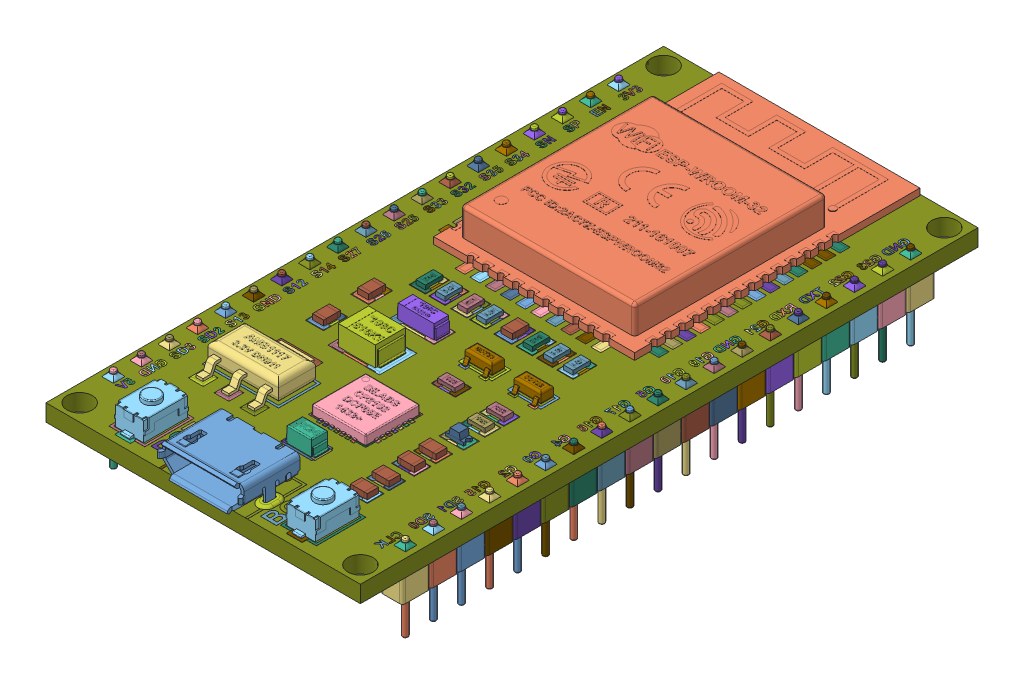
SolidWorks assembly PCB_ESP32-38Pines, configuration Default. Lengths in mm.
Overall size (28 10.12 55.48).
487 component instances, 472 part files, 0 mates.
Components (placement in the parent):
- PCB_ESP32-38Pines.step-1: PCB_ESP32-38Pines.step [Default] at origin size (28 10.12 55.48)
  - MicroUSB.step-1: MicroUSB.step [Default] at (0 2.6382 22.5) size (7.56 3.45 5.78)
  - esp32.step-1: esp32.step [Default] at (0 1.5 -14.6737) size (17.9 3.13 25.4)
  - AMS1173.3V.step-1: AMS1173.3V.step [Default] at (-6.6341 1.5 15.6567) x (-1 0 0) z (0 0 -1) size (6.3 1.81 6.45)
  - cp2102.step-1: cp2102.step [Default] at (1.1401 1.501 14.1651) x (1 0 0) z (0 1 0) size (5.1 5.1 0.81)
  - Push_Bottom.step-1: Push_Bottom.step [Default] at (-7.7988 1.5 24.2992) x (0 0 -1) z (1 0 0) size (4.7 2.2 2.7)
  - Push_Bottom.step-2: Push_Bottom.step [Default] at (7.4774 1.5 24.2992) x (0 0 -1) z (1 0 0) size (4.7 2.2 2.7)
  - Diodo_K24.step-1: Diodo_K24.step [Default] at (0.9466 1.5 19.1832) size (2.7 1.4 1.4)
  - Cap_Tam_106.step-1: Cap_Tam_106.step [Default] at (-3.6422 1.5 8.8277) size (3.8 1.81 2.7)
  - Cap_Tam_106C.step-1: Cap_Tam_106C.step [Default] at (-3.1152 1.5 4.7703) size (3.5 1.31 1.3)
  - Transistor_smd.step-1: Transistor_smd.step [Default] at (7.0469 1.5 5.1079) size (2.4 1.01 2)
  - Transistor_smd.step-2: Transistor_smd.step [Default] at (2.6755 1.5 5.1079) size (2.4 1.01 2)
  - Led_red_0603.step-1: Led_red_0603.step [Default] at (7.1609 1.5 11.8696) size (1.6 0.85 0.8)
  - Cap_0603.step-1: Cap_0603.step [Default] at (7.0673 1.5 14.1024) x (1 0 0) z (0 1 0) size (1.5 1 0.5)
  - Cap_0603.step-2: Cap_0603.step [Default] at (7.0673 1.5 16.0214) x (1 0 0) z (0 1 0) size (1.5 1 0.5)
  - Cap_0603.step-3: Cap_0603.step [Default] at (7.0673 1.5 18.2661) x (1 0 0) z (0 1 0) size (1.5 1 0.5)
  - Cap_0603.step-4: Cap_0603.step [Default] at (7.0673 2 20.2101) x (1 0 0) z (0 -1 0) size (1.5 1 0.5)
  - Res_102.step-1: Res_102.step [Default] at (7.1297 1.7 10.3267) x (-1 0 0) z (0 -1 0) size (1.55 0.85 0.41)
  - Res_123.step-1: Res_123.step [Default] at (7.1297 1.7 8.6342) x (-1 0 0) z (0 -1 0) size (1.55 0.85 0.41)
  - Res_123.step-2: Res_123.step [Default] at (2.693 1.7 8.548) x (-1 0 0.000044) z (0 -1 0) size (1.55 0.85 0.41)
  - Res_471.step-1: Res_471.step [Default] at (7.366 1.7 1.1543) x (0 0 1) z (0 -1 0) size (1.55 0.85 0.41)
  - Res_471.step-2: Res_471.step [Default] at (5.5706 1.7 1.1543) x (0 0 1) z (0 -1 0) size (1.55 0.85 0.41)
  - Res_471.step-3: Res_471.step [Default] at (-0.3842 1.7 1.1543) x (0 0 1) z (0 -1 0) size (1.55 0.85 0.41)
  - Res_471.step-4: Res_471.step [Default] at (-4.0229 1.7 1.1543) x (0 0 1) z (0 -1 0) size (1.55 0.85 0.41)
  - Res_123.step-3: Res_123.step [Default] at (-2.9307 1.7 1.1543) x (0 0 -1) z (0 -1 0) size (1.55 0.85 0.41)
  - Res_512.step-1: Res_512.step [Default] at (2.8915 1.7 1.1543) x (0 0 -1) z (0 -1 0) size (1.55 0.85 0.41)
  - Res_512.step-2: Res_512.step [Default] at (-6.6341 1.7 1.1543) x (0 0 -1) z (0 -1 0) size (1.55 0.85 0.41)
  - Cap_0603.step-5: Cap_0603.step [Default] at (1.4432 2 1.1648) x (0 0 -1) z (0 -1 0) size (1.5 1 0.5)
  - Cap_0603.step-6: Cap_0603.step [Default] at (-8.012 2 4.503) x (0 0 -1) z (0 -1 0) size (1.5 1 0.5)
  - Cap_0603.step-7: Cap_0603.step [Default] at (-8.012 2 8.5113) x (0 0 -1) z (0 -1 0) size (1.5 1 0.5)
  - PCB_ESP32-38Pines (v2~recovered).step-1: PCB_ESP32-38Pines (v2~recovered).step [Default] at origin size (28 1.5 55)
  - PCB_ESP32-38Pines (v2~recovered)-0.step-1: PCB_ESP32-38Pines (v2~recovered)-0.step [Default] at origin size (0.5 0.65 0.5)
  - PCB_ESP32-38Pines (v2~recovered)-1.step-1: PCB_ESP32-38Pines (v2~recovered)-1.step [Default] at origin size (0.5 0.65 0.5)
  - PCB_ESP32-38Pines (v2~recovered)-2.step-1: PCB_ESP32-38Pines (v2~recovered)-2.step [Default] at origin size (0.5 0.65 0.5)
  - PCB_ESP32-38Pines (v2~recovered)-3.step-1: PCB_ESP32-38Pines (v2~recovered)-3.step [Default] at origin size (0.5 0.65 0.5)
  - PCB_ESP32-38Pines (v2~recovered)-4.step-1: PCB_ESP32-38Pines (v2~recovered)-4.step [Default] at origin size (0.5 0.65 0.5)
  - PCB_ESP32-38Pines (v2~recovered)-5.step-1: PCB_ESP32-38Pines (v2~recovered)-5.step [Default] at origin size (0.5 0.65 0.5)
  - PCB_ESP32-38Pines (v2~recovered)-6.step-1: PCB_ESP32-38Pines (v2~recovered)-6.step [Default] at origin size (0.5 0.65 0.5)
  - PCB_ESP32-38Pines (v2~recovered)-7.step-1: PCB_ESP32-38Pines (v2~recovered)-7.step [Default] at origin size (0.5 0.65 0.5)
  - PCB_ESP32-38Pines (v2~recovered)-8.step-1: PCB_ESP32-38Pines (v2~recovered)-8.step [Default] at origin size (0.5 0.65 0.5)
  - PCB_ESP32-38Pines (v2~recovered)-9.step-1: PCB_ESP32-38Pines (v2~recovered)-9.step [Default] at origin size (0.5 0.65 0.5)
  - PCB_ESP32-38Pines (v2~recovered)-10.step-1: PCB_ESP32-38Pines (v2~recovered)-10.step [Default] at origin size (0.5 0.65 0.5)
  - PCB_ESP32-38Pines (v2~recovered)-11.step-1: PCB_ESP32-38Pines (v2~recovered)-11.step [Default] at origin size (0.5 0.65 0.5)
  - PCB_ESP32-38Pines (v2~recovered)-12.step-1: PCB_ESP32-38Pines (v2~recovered)-12.step [Default] at origin size (0.5 0.65 0.5)
  - PCB_ESP32-38Pines (v2~recovered)-13.step-1: PCB_ESP32-38Pines (v2~recovered)-13.step [Default] at origin size (0.5 0.65 0.5)
  - PCB_ESP32-38Pines (v2~recovered)-14.step-1: PCB_ESP32-38Pines (v2~recovered)-14.step [Default] at origin size (0.5 0.65 0.5)
  - PCB_ESP32-38Pines (v2~recovered)-15.step-1: PCB_ESP32-38Pines (v2~recovered)-15.step [Default] at origin size (0.5 0.65 0.5)
  - PCB_ESP32-38Pines (v2~recovered)-16.step-1: PCB_ESP32-38Pines (v2~recovered)-16.step [Default] at origin size (0.5 0.65 0.5)
  - PCB_ESP32-38Pines (v2~recovered)-17.step-1: PCB_ESP32-38Pines (v2~recovered)-17.step [Default] at origin size (0.5 0.65 0.5)
  - PCB_ESP32-38Pines (v2~recovered)-18.step-1: PCB_ESP32-38Pines (v2~recovered)-18.step [Default] at origin size (0.5 0.65 0.5)
  - PCB_ESP32-38Pines (v2~recovered)-19.step-1: PCB_ESP32-38Pines (v2~recovered)-19.step [Default] at origin size (0.5 0.65 0.5)
  - PCB_ESP32-38Pines (v2~recovered)-20.step-1: PCB_ESP32-38Pines (v2~recovered)-20.step [Default] at origin size (0.5 0.65 0.5)
  - PCB_ESP32-38Pines (v2~recovered)-21.step-1: PCB_ESP32-38Pines (v2~recovered)-21.step [Default] at origin size (0.5 0.65 0.5)
  - PCB_ESP32-38Pines (v2~recovered)-22.step-1: PCB_ESP32-38Pines (v2~recovered)-22.step [Default] at origin size (0.5 0.65 0.5)
  - PCB_ESP32-38Pines (v2~recovered)-23.step-1: PCB_ESP32-38Pines (v2~recovered)-23.step [Default] at origin size (0.5 0.65 0.5)
  - PCB_ESP32-38Pines (v2~recovered)-24.step-1: PCB_ESP32-38Pines (v2~recovered)-24.step [Default] at origin size (0.5 0.65 0.5)
  - PCB_ESP32-38Pines (v2~recovered)-25.step-1: PCB_ESP32-38Pines (v2~recovered)-25.step [Default] at origin size (0.5 0.65 0.5)
  - PCB_ESP32-38Pines (v2~recovered)-26.step-1: PCB_ESP32-38Pines (v2~recovered)-26.step [Default] at origin size (0.5 0.65 0.5)
  - PCB_ESP32-38Pines (v2~recovered)-27.step-1: PCB_ESP32-38Pines (v2~recovered)-27.step [Default] at origin size (0.5 0.65 0.5)
  - PCB_ESP32-38Pines (v2~recovered)-28.step-1: PCB_ESP32-38Pines (v2~recovered)-28.step [Default] at origin size (0.5 0.65 0.5)
  - PCB_ESP32-38Pines (v2~recovered)-29.step-1: PCB_ESP32-38Pines (v2~recovered)-29.step [Default] at origin size (0.5 0.65 0.5)
  - PCB_ESP32-38Pines (v2~recovered)-30.step-1: PCB_ESP32-38Pines (v2~recovered)-30.step [Default] at origin size (0.5 0.65 0.5)
  - PCB_ESP32-38Pines (v2~recovered)-31.step-1: PCB_ESP32-38Pines (v2~recovered)-31.step [Default] at origin size (0.5 0.65 0.5)
  - PCB_ESP32-38Pines (v2~recovered)-32.step-1: PCB_ESP32-38Pines (v2~recovered)-32.step [Default] at origin size (0.5 0.65 0.5)
  - PCB_ESP32-38Pines (v2~recovered)-33.step-1: PCB_ESP32-38Pines (v2~recovered)-33.step [Default] at origin size (0.5 0.65 0.5)
  - PCB_ESP32-38Pines (v2~recovered)-34.step-1: PCB_ESP32-38Pines (v2~recovered)-34.step [Default] at origin size (0.5 0.65 0.5)
  - PCB_ESP32-38Pines (v2~recovered)-35.step-1: PCB_ESP32-38Pines (v2~recovered)-35.step [Default] at origin size (0.5 0.65 0.5)
  - PCB_ESP32-38Pines (v2~recovered)-36.step-1: PCB_ESP32-38Pines (v2~recovered)-36.step [Default] at origin size (0.5 0.65 0.5)
  - PCB_ESP32-38Pines (v2~recovered)-37.step-1: PCB_ESP32-38Pines (v2~recovered)-37.step [Default] at origin size (0.5 0.65 0.5)
  - PCB_ESP32-38Pines (v2~recovered)-38.step-1: PCB_ESP32-38Pines (v2~recovered)-38.step [Default] at origin size (0.5 7 0.5)
  - PCB_ESP32-38Pines (v2~recovered)-39.step-1: PCB_ESP32-38Pines (v2~recovered)-39.step [Default] at origin size (0.5 7 0.5)
  - PCB_ESP32-38Pines (v2~recovered)-40.step-1: PCB_ESP32-38Pines (v2~recovered)-40.step [Default] at origin size (0.5 7 0.5)
  - PCB_ESP32-38Pines (v2~recovered)-41.step-1: PCB_ESP32-38Pines (v2~recovered)-41.step [Default] at origin size (0.5 7 0.5)
  - PCB_ESP32-38Pines (v2~recovered)-42.step-1: PCB_ESP32-38Pines (v2~recovered)-42.step [Default] at origin size (0.5 7 0.5)
  - PCB_ESP32-38Pines (v2~recovered)-43.step-1: PCB_ESP32-38Pines (v2~recovered)-43.step [Default] at origin size (0.5 7 0.5)
  - PCB_ESP32-38Pines (v2~recovered)-44.step-1: PCB_ESP32-38Pines (v2~recovered)-44.step [Default] at origin size (0.5 7 0.5)
  - PCB_ESP32-38Pines (v2~recovered)-45.step-1: PCB_ESP32-38Pines (v2~recovered)-45.step [Default] at origin size (0.5 7 0.5)
  - PCB_ESP32-38Pines (v2~recovered)-46.step-1: PCB_ESP32-38Pines (v2~recovered)-46.step [Default] at origin size (0.5 7 0.5)
  - PCB_ESP32-38Pines (v2~recovered)-47.step-1: PCB_ESP32-38Pines (v2~recovered)-47.step [Default] at origin size (0.5 7 0.5)
  - PCB_ESP32-38Pines (v2~recovered)-48.step-1: PCB_ESP32-38Pines (v2~recovered)-48.step [Default] at origin size (0.5 7 0.5)
  - PCB_ESP32-38Pines (v2~recovered)-49.step-1: PCB_ESP32-38Pines (v2~recovered)-49.step [Default] at origin size (0.5 7 0.5)
  - PCB_ESP32-38Pines (v2~recovered)-50.step-1: PCB_ESP32-38Pines (v2~recovered)-50.step [Default] at origin size (0.5 7 0.5)
  - PCB_ESP32-38Pines (v2~recovered)-51.step-1: PCB_ESP32-38Pines (v2~recovered)-51.step [Default] at origin size (0.5 7 0.5)
  - PCB_ESP32-38Pines (v2~recovered)-52.step-1: PCB_ESP32-38Pines (v2~recovered)-52.step [Default] at origin size (0.5 7 0.5)
  - PCB_ESP32-38Pines (v2~recovered)-53.step-1: PCB_ESP32-38Pines (v2~recovered)-53.step [Default] at origin size (0.5 7 0.5)
  - PCB_ESP32-38Pines (v2~recovered)-54.step-1: PCB_ESP32-38Pines (v2~recovered)-54.step [Default] at origin size (0.5 7 0.5)
  - PCB_ESP32-38Pines (v2~recovered)-55.step-1: PCB_ESP32-38Pines (v2~recovered)-55.step [Default] at origin size (0.5 7 0.5)
  - PCB_ESP32-38Pines (v2~recovered)-56.step-1: PCB_ESP32-38Pines (v2~recovered)-56.step [Default] at origin size (0.5 7 0.5)
  - PCB_ESP32-38Pines (v2~recovered)-57.step-1: PCB_ESP32-38Pines (v2~recovered)-57.step [Default] at origin size (0.5 7 0.5)
  - PCB_ESP32-38Pines (v2~recovered)-58.step-1: PCB_ESP32-38Pines (v2~recovered)-58.step [Default] at origin size (0.5 7 0.5)
  - PCB_ESP32-38Pines (v2~recovered)-59.step-1: PCB_ESP32-38Pines (v2~recovered)-59.step [Default] at origin size (0.5 7 0.5)
  - PCB_ESP32-38Pines (v2~recovered)-60.step-1: PCB_ESP32-38Pines (v2~recovered)-60.step [Default] at origin size (0.5 7 0.5)
  - PCB_ESP32-38Pines (v2~recovered)-61.step-1: PCB_ESP32-38Pines (v2~recovered)-61.step [Default] at origin size (0.5 7 0.5)
  - PCB_ESP32-38Pines (v2~recovered)-62.step-1: PCB_ESP32-38Pines (v2~recovered)-62.step [Default] at origin size (0.5 7 0.5)
  - PCB_ESP32-38Pines (v2~recovered)-63.step-1: PCB_ESP32-38Pines (v2~recovered)-63.step [Default] at origin size (0.5 7 0.5)
  - PCB_ESP32-38Pines (v2~recovered)-64.step-1: PCB_ESP32-38Pines (v2~recovered)-64.step [Default] at origin size (0.5 7 0.5)
  - PCB_ESP32-38Pines (v2~recovered)-65.step-1: PCB_ESP32-38Pines (v2~recovered)-65.step [Default] at origin size (0.5 7 0.5)
  - PCB_ESP32-38Pines (v2~recovered)-66.step-1: PCB_ESP32-38Pines (v2~recovered)-66.step [Default] at origin size (0.5 7 0.5)
  - PCB_ESP32-38Pines (v2~recovered)-67.step-1: PCB_ESP32-38Pines (v2~recovered)-67.step [Default] at origin size (0.5 7 0.5)
  - PCB_ESP32-38Pines (v2~recovered)-68.step-1: PCB_ESP32-38Pines (v2~recovered)-68.step [Default] at origin size (0.5 7 0.5)
  - PCB_ESP32-38Pines (v2~recovered)-69.step-1: PCB_ESP32-38Pines (v2~recovered)-69.step [Default] at origin size (0.5 7 0.5)
  - PCB_ESP32-38Pines (v2~recovered)-70.step-1: PCB_ESP32-38Pines (v2~recovered)-70.step [Default] at origin size (0.5 7 0.5)
  - PCB_ESP32-38Pines (v2~recovered)-71.step-1: PCB_ESP32-38Pines (v2~recovered)-71.step [Default] at origin size (0.5 7 0.5)
  - PCB_ESP32-38Pines (v2~recovered)-72.step-1: PCB_ESP32-38Pines (v2~recovered)-72.step [Default] at origin size (0.5 7 0.5)
  - PCB_ESP32-38Pines (v2~recovered)-73.step-1: PCB_ESP32-38Pines (v2~recovered)-73.step [Default] at origin size (0.5 7 0.5)
  - PCB_ESP32-38Pines (v2~recovered)-74.step-1: PCB_ESP32-38Pines (v2~recovered)-74.step [Default] at origin size (0.5 7 0.5)
  - PCB_ESP32-38Pines (v2~recovered)-75.step-1: PCB_ESP32-38Pines (v2~recovered)-75.step [Default] at origin size (0.5 7 0.5)
  - PCB_ESP32-38Pines (v2~recovered)-76.step-1: PCB_ESP32-38Pines (v2~recovered)-76.step [Default] at origin size (2 2 2.5)
  - PCB_ESP32-38Pines (v2~recovered)-77.step-1: PCB_ESP32-38Pines (v2~recovered)-77.step [Default] at origin size (2 2 2.5)
  - PCB_ESP32-38Pines (v2~recovered)-78.step-1: PCB_ESP32-38Pines (v2~recovered)-78.step [Default] at origin size (2 2 2.5)
  - PCB_ESP32-38Pines (v2~recovered)-79.step-1: PCB_ESP32-38Pines (v2~recovered)-79.step [Default] at origin size (2 2 2.5)
  - PCB_ESP32-38Pines (v2~recovered)-80.step-1: PCB_ESP32-38Pines (v2~recovered)-80.step [Default] at origin size (2 2 2.5)
  - PCB_ESP32-38Pines (v2~recovered)-81.step-1: PCB_ESP32-38Pines (v2~recovered)-81.step [Default] at origin size (2 2 2.5)
  - PCB_ESP32-38Pines (v2~recovered)-82.step-1: PCB_ESP32-38Pines (v2~recovered)-82.step [Default] at origin size (2 2 2.5)
  - PCB_ESP32-38Pines (v2~recovered)-83.step-1: PCB_ESP32-38Pines (v2~recovered)-83.step [Default] at origin size (2 2 2.5)
  - PCB_ESP32-38Pines (v2~recovered)-84.step-1: PCB_ESP32-38Pines (v2~recovered)-84.step [Default] at origin size (2 2 2.5)
  - PCB_ESP32-38Pines (v2~recovered)-85.step-1: PCB_ESP32-38Pines (v2~recovered)-85.step [Default] at origin size (2 2 2.5)
  - PCB_ESP32-38Pines (v2~recovered)-86.step-1: PCB_ESP32-38Pines (v2~recovered)-86.step [Default] at origin size (2 2 2.5)
  - PCB_ESP32-38Pines (v2~recovered)-87.step-1: PCB_ESP32-38Pines (v2~recovered)-87.step [Default] at origin size (2 2 2.5)
  - PCB_ESP32-38Pines (v2~recovered)-88.step-1: PCB_ESP32-38Pines (v2~recovered)-88.step [Default] at origin size (2 2 2.5)
  - PCB_ESP32-38Pines (v2~recovered)-89.step-1: PCB_ESP32-38Pines (v2~recovered)-89.step [Default] at origin size (2 2 2.5)
  - PCB_ESP32-38Pines (v2~recovered)-90.step-1: PCB_ESP32-38Pines (v2~recovered)-90.step [Default] at origin size (2 2 2.5)
  - PCB_ESP32-38Pines (v2~recovered)-91.step-1: PCB_ESP32-38Pines (v2~recovered)-91.step [Default] at origin size (2 2 2.5)
  - PCB_ESP32-38Pines (v2~recovered)-92.step-1: PCB_ESP32-38Pines (v2~recovered)-92.step [Default] at origin size (2 2 2.5)
  - PCB_ESP32-38Pines (v2~recovered)-93.step-1: PCB_ESP32-38Pines (v2~recovered)-93.step [Default] at origin size (2 2 2.5)
  - PCB_ESP32-38Pines (v2~recovered)-94.step-1: PCB_ESP32-38Pines (v2~recovered)-94.step [Default] at origin size (2 2 2.5)
  - PCB_ESP32-38Pines (v2~recovered)-95.step-1: PCB_ESP32-38Pines (v2~recovered)-95.step [Default] at origin size (2 2 2.5)
  - PCB_ESP32-38Pines (v2~recovered)-96.step-1: PCB_ESP32-38Pines (v2~recovered)-96.step [Default] at origin size (2 2 2.5)
  - PCB_ESP32-38Pines (v2~recovered)-97.step-1: PCB_ESP32-38Pines (v2~recovered)-97.step [Default] at origin size (2 2 2.5)
  - PCB_ESP32-38Pines (v2~recovered)-98.step-1: PCB_ESP32-38Pines (v2~recovered)-98.step [Default] at origin size (2 2 2.5)
  - PCB_ESP32-38Pines (v2~recovered)-99.step-1: PCB_ESP32-38Pines (v2~recovered)-99.step [Default] at origin size (2 2 2.5)
  - PCB_ESP32-38Pines (v2~recovered)-100.step-1: PCB_ESP32-38Pines (v2~recovered)-100.step [Default] at origin size (2 2 2.5)
  - PCB_ESP32-38Pines (v2~recovered)-101.step-1: PCB_ESP32-38Pines (v2~recovered)-101.step [Default] at origin size (2 2 2.5)
  - PCB_ESP32-38Pines (v2~recovered)-102.step-1: PCB_ESP32-38Pines (v2~recovered)-102.step [Default] at origin size (2 2 2.5)
  - PCB_ESP32-38Pines (v2~recovered)-103.step-1: PCB_ESP32-38Pines (v2~recovered)-103.step [Default] at origin size (2 2 2.5)
  - PCB_ESP32-38Pines (v2~recovered)-104.step-1: PCB_ESP32-38Pines (v2~recovered)-104.step [Default] at origin size (2 2 2.5)
  - PCB_ESP32-38Pines (v2~recovered)-105.step-1: PCB_ESP32-38Pines (v2~recovered)-105.step [Default] at origin size (2 2 2.5)
  - PCB_ESP32-38Pines (v2~recovered)-106.step-1: PCB_ESP32-38Pines (v2~recovered)-106.step [Default] at origin size (2 2 2.5)
  - PCB_ESP32-38Pines (v2~recovered)-107.step-1: PCB_ESP32-38Pines (v2~recovered)-107.step [Default] at origin size (2 2 2.5)
  - PCB_ESP32-38Pines (v2~recovered)-108.step-1: PCB_ESP32-38Pines (v2~recovered)-108.step [Default] at origin size (2 2 2.5)
  - PCB_ESP32-38Pines (v2~recovered)-109.step-1: PCB_ESP32-38Pines (v2~recovered)-109.step [Default] at origin size (2 2 2.5)
  - PCB_ESP32-38Pines (v2~recovered)-110.step-1: PCB_ESP32-38Pines (v2~recovered)-110.step [Default] at origin size (2 2 2.5)
  - PCB_ESP32-38Pines (v2~recovered)-111.step-1: PCB_ESP32-38Pines (v2~recovered)-111.step [Default] at origin size (2 2 2.5)
  - PCB_ESP32-38Pines (v2~recovered)-112.step-1: PCB_ESP32-38Pines (v2~recovered)-112.step [Default] at origin size (2 2 2.5)
  - PCB_ESP32-38Pines (v2~recovered)-113.step-1: PCB_ESP32-38Pines (v2~recovered)-113.step [Default] at origin size (2 2 2.5)
  - PCB_ESP32-38Pines (v2~recovered)-114.step-1: PCB_ESP32-38Pines (v2~recovered)-114.step [Default] at origin size (1 0.41 1)
  - PCB_ESP32-38Pines (v2~recovered)-115.step-1: PCB_ESP32-38Pines (v2~recovered)-115.step [Default] at origin size (1 0.41 1)
  - PCB_ESP32-38Pines (v2~recovered)-116.step-1: PCB_ESP32-38Pines (v2~recovered)-116.step [Default] at origin size (1 0.41 1)
  - PCB_ESP32-38Pines (v2~recovered)-117.step-1: PCB_ESP32-38Pines (v2~recovered)-117.step [Default] at origin size (1 0.41 1)
  - PCB_ESP32-38Pines (v2~recovered)-118.step-1: PCB_ESP32-38Pines (v2~recovered)-118.step [Default] at origin size (1 0.41 1)
  - PCB_ESP32-38Pines (v2~recovered)-119.step-1: PCB_ESP32-38Pines (v2~recovered)-119.step [Default] at origin size (1 0.41 1)
  - PCB_ESP32-38Pines (v2~recovered)-120.step-1: PCB_ESP32-38Pines (v2~recovered)-120.step [Default] at origin size (1 0.41 1)
  - PCB_ESP32-38Pines (v2~recovered)-121.step-1: PCB_ESP32-38Pines (v2~recovered)-121.step [Default] at origin size (1 0.41 1)
  - PCB_ESP32-38Pines (v2~recovered)-122.step-1: PCB_ESP32-38Pines (v2~recovered)-122.step [Default] at origin size (1 0.41 1)
  - PCB_ESP32-38Pines (v2~recovered)-123.step-1: PCB_ESP32-38Pines (v2~recovered)-123.step [Default] at origin size (1 0.41 1)
  - PCB_ESP32-38Pines (v2~recovered)-124.step-1: PCB_ESP32-38Pines (v2~recovered)-124.step [Default] at origin size (1 0.41 1)
  - PCB_ESP32-38Pines (v2~recovered)-125.step-1: PCB_ESP32-38Pines (v2~recovered)-125.step [Default] at origin size (1 0.41 1)
  - PCB_ESP32-38Pines (v2~recovered)-126.step-1: PCB_ESP32-38Pines (v2~recovered)-126.step [Default] at origin size (1 0.41 1)
  - PCB_ESP32-38Pines (v2~recovered)-127.step-1: PCB_ESP32-38Pines (v2~recovered)-127.step [Default] at origin size (1 0.41 1)
  - PCB_ESP32-38Pines (v2~recovered)-128.step-1: PCB_ESP32-38Pines (v2~recovered)-128.step [Default] at origin size (1 0.41 1)
  - PCB_ESP32-38Pines (v2~recovered)-129.step-1: PCB_ESP32-38Pines (v2~recovered)-129.step [Default] at origin size (1 0.41 1)
  - PCB_ESP32-38Pines (v2~recovered)-130.step-1: PCB_ESP32-38Pines (v2~recovered)-130.step [Default] at origin size (1 0.41 1)
  - PCB_ESP32-38Pines (v2~recovered)-131.step-1: PCB_ESP32-38Pines (v2~recovered)-131.step [Default] at origin size (1 0.41 1)
  - PCB_ESP32-38Pines (v2~recovered)-132.step-1: PCB_ESP32-38Pines (v2~recovered)-132.step [Default] at origin size (1 0.41 1)
  - PCB_ESP32-38Pines (v2~recovered)-133.step-1: PCB_ESP32-38Pines (v2~recovered)-133.step [Default] at origin size (1 0.41 1)
  - PCB_ESP32-38Pines (v2~recovered)-134.step-1: PCB_ESP32-38Pines (v2~recovered)-134.step [Default] at origin size (1 0.41 1)
  - PCB_ESP32-38Pines (v2~recovered)-135.step-1: PCB_ESP32-38Pines (v2~recovered)-135.step [Default] at origin size (1 0.41 1)
  - PCB_ESP32-38Pines (v2~recovered)-136.step-1: PCB_ESP32-38Pines (v2~recovered)-136.step [Default] at origin size (1 0.41 1)
  - PCB_ESP32-38Pines (v2~recovered)-137.step-1: PCB_ESP32-38Pines (v2~recovered)-137.step [Default] at origin size (1 0.41 1)
  - PCB_ESP32-38Pines (v2~recovered)-138.step-1: PCB_ESP32-38Pines (v2~recovered)-138.step [Default] at origin size (1 0.41 1)
  - PCB_ESP32-38Pines (v2~recovered)-139.step-1: PCB_ESP32-38Pines (v2~recovered)-139.step [Default] at origin size (1 0.41 1)
  - PCB_ESP32-38Pines (v2~recovered)-140.step-1: PCB_ESP32-38Pines (v2~recovered)-140.step [Default] at origin size (1 0.41 1)
  - PCB_ESP32-38Pines (v2~recovered)-141.step-1: PCB_ESP32-38Pines (v2~recovered)-141.step [Default] at origin size (1 0.41 1)
  - PCB_ESP32-38Pines (v2~recovered)-142.step-1: PCB_ESP32-38Pines (v2~recovered)-142.step [Default] at origin size (1 0.41 1)
  - PCB_ESP32-38Pines (v2~recovered)-143.step-1: PCB_ESP32-38Pines (v2~recovered)-143.step [Default] at origin size (1 0.41 1)
  - PCB_ESP32-38Pines (v2~recovered)-144.step-1: PCB_ESP32-38Pines (v2~recovered)-144.step [Default] at origin size (1 0.41 1)
  - PCB_ESP32-38Pines (v2~recovered)-145.step-1: PCB_ESP32-38Pines (v2~recovered)-145.step [Default] at origin size (1 0.41 1)
  - PCB_ESP32-38Pines (v2~recovered)-146.step-1: PCB_ESP32-38Pines (v2~recovered)-146.step [Default] at origin size (1 0.41 1)
  - PCB_ESP32-38Pines (v2~recovered)-147.step-1: PCB_ESP32-38Pines (v2~recovered)-147.step [Default] at origin size (1 0.41 1)
  - PCB_ESP32-38Pines (v2~recovered)-148.step-1: PCB_ESP32-38Pines (v2~recovered)-148.step [Default] at origin size (1 0.41 1)
  - PCB_ESP32-38Pines (v2~recovered)-149.step-1: PCB_ESP32-38Pines (v2~recovered)-149.step [Default] at origin size (1 0.41 1)
  - PCB_ESP32-38Pines (v2~recovered)-150.step-1: PCB_ESP32-38Pines (v2~recovered)-150.step [Default] at origin size (1 0.41 1)
  - PCB_ESP32-38Pines (v2~recovered)-151.step-1: PCB_ESP32-38Pines (v2~recovered)-151.step [Default] at origin size (1 0.41 1)
  - PCB_ESP32-38Pines (v2~recovered)-152.step-1: PCB_ESP32-38Pines (v2~recovered)-152.step [Default] at origin size (1.6 0.01 2.15)
  - PCB_ESP32-38Pines (v2~recovered)-153.step-1: PCB_ESP32-38Pines (v2~recovered)-153.step [Default] at origin size (2.15 0.01 1.45)
  - PCB_ESP32-38Pines (v2~recovered)-154.step-1: PCB_ESP32-38Pines (v2~recovered)-154.step [Default] at origin size (1.45 0.01 2.15)
  - PCB_ESP32-38Pines (v2~recovered)-155.step-1: PCB_ESP32-38Pines (v2~recovered)-155.step [Default] at origin size (1.45 0.01 2.15)
  - PCB_ESP32-38Pines (v2~recovered)-156.step-1: PCB_ESP32-38Pines (v2~recovered)-156.step [Default] at origin size (0.67 0.01 0.58)
  - PCB_ESP32-38Pines (v2~recovered)-157.step-1: PCB_ESP32-38Pines (v2~recovered)-157.step [Default] at origin size (1.99 0.01 1.5)
  - PCB_ESP32-38Pines (v2~recovered)-158.step-1: PCB_ESP32-38Pines (v2~recovered)-158.step [Default] at origin size (0.83 0.01 0.83)
  - PCB_ESP32-38Pines (v2~recovered)-159.step-1: PCB_ESP32-38Pines (v2~recovered)-159.step [Default] at origin size (2 0.01 1.5)
  - PCB_ESP32-38Pines (v2~recovered)-160.step-1: PCB_ESP32-38Pines (v2~recovered)-160.step [Default] at origin size (3.2 0.01 4.4)
  - PCB_ESP32-38Pines (v2~recovered)-161.step-1: PCB_ESP32-38Pines (v2~recovered)-161.step [Default] at origin size (0.83 0.01 0.83)
  - PCB_ESP32-38Pines (v2~recovered)-162.step-1: PCB_ESP32-38Pines (v2~recovered)-162.step [Default] at origin size (2 0.01 1.5)
  - PCB_ESP32-38Pines (v2~recovered)-163.step-1: PCB_ESP32-38Pines (v2~recovered)-163.step [Default] at origin size (2.1 0.01 5.3)
  - PCB_ESP32-38Pines (v2~recovered)-164.step-1: PCB_ESP32-38Pines (v2~recovered)-164.step [Default] at origin size (1.45 0.01 2.15)
  - PCB_ESP32-38Pines (v2~recovered)-165.step-1: PCB_ESP32-38Pines (v2~recovered)-165.step [Default] at origin size (1.45 0.01 2.15)
  - PCB_ESP32-38Pines (v2~recovered)-166.step-1: PCB_ESP32-38Pines (v2~recovered)-166.step [Default] at origin size (3.8 0.01 1.9)
  - PCB_ESP32-38Pines (v2~recovered)-167.step-1: PCB_ESP32-38Pines (v2~recovered)-167.step [Default] at origin size (1.6 0.01 2.15)
  - PCB_ESP32-38Pines (v2~recovered)-168.step-1: PCB_ESP32-38Pines (v2~recovered)-168.step [Default] at origin size (2.15 0.01 1.45)
  - PCB_ESP32-38Pines (v2~recovered)-169.step-1: PCB_ESP32-38Pines (v2~recovered)-169.step [Default] at origin size (2.15 0.01 1.45)
  - PCB_ESP32-38Pines (v2~recovered)-170.step-1: PCB_ESP32-38Pines (v2~recovered)-170.step [Default] at origin size (3 0.01 1.7)
  - PCB_ESP32-38Pines (v2~recovered)-171.step-1: PCB_ESP32-38Pines (v2~recovered)-171.step [Default] at origin size (1.6 0.01 2.15)
  - PCB_ESP32-38Pines (v2~recovered)-172.step-1: PCB_ESP32-38Pines (v2~recovered)-172.step [Default] at origin size (1.45 0.01 2.15)
  - PCB_ESP32-38Pines (v2~recovered)-173.step-1: PCB_ESP32-38Pines (v2~recovered)-173.step [Default] at origin size (2.7 0.01 1.9)
  - PCB_ESP32-38Pines (v2~recovered)-174.step-1: PCB_ESP32-38Pines (v2~recovered)-174.step [Default] at origin size (0.83 0.01 0.83)
  - PCB_ESP32-38Pines (v2~recovered)-175.step-1: PCB_ESP32-38Pines (v2~recovered)-175.step [Default] at origin size (2 0.01 1.5)
  - PCB_ESP32-38Pines (v2~recovered)-176.step-1: PCB_ESP32-38Pines (v2~recovered)-176.step [Default] at origin size (3.2 0.01 4.4)
  - PCB_ESP32-38Pines (v2~recovered)-177.step-1: PCB_ESP32-38Pines (v2~recovered)-177.step [Default] at origin size (6.8 0.01 3.8)
  - PCB_ESP32-38Pines (v2~recovered)-178.step-1: PCB_ESP32-38Pines (v2~recovered)-178.step [Default] at origin size (0.83 0.01 0.81)
  - PCB_ESP32-38Pines (v2~recovered)-179.step-1: PCB_ESP32-38Pines (v2~recovered)-179.step [Default] at origin size (2.08 0.01 5.3)
  - PCB_ESP32-38Pines (v2~recovered)-180.step-1: PCB_ESP32-38Pines (v2~recovered)-180.step [Default] at origin size (1.45 0.01 2.15)
  - PCB_ESP32-38Pines (v2~recovered)-181.step-1: PCB_ESP32-38Pines (v2~recovered)-181.step [Default] at origin size (1.45 0.01 2.15)
  - PCB_ESP32-38Pines (v2~recovered)-182.step-1: PCB_ESP32-38Pines (v2~recovered)-182.step [Default] at origin size (3 0.01 1.7)
  - PCB_ESP32-38Pines (v2~recovered)-183.step-1: PCB_ESP32-38Pines (v2~recovered)-183.step [Default] at origin size (3.9 0.01 3.3)
  - PCB_ESP32-38Pines (v2~recovered)-184.step-1: PCB_ESP32-38Pines (v2~recovered)-184.step [Default] at origin size (2.2 0.01 1.4)
  - PCB_ESP32-38Pines (v2~recovered)-185.step-1: PCB_ESP32-38Pines (v2~recovered)-185.step [Default] at origin size (0.72 0.01 0.6)
  - PCB_ESP32-38Pines (v2~recovered)-186.step-1: PCB_ESP32-38Pines (v2~recovered)-186.step [Default] at origin size (0.72 0.01 0.6)
  - PCB_ESP32-38Pines (v2~recovered)-187.step-1: PCB_ESP32-38Pines (v2~recovered)-187.step [Default] at origin size (0.72 0.01 0.48)
  - PCB_ESP32-38Pines (v2~recovered)-188.step-1: PCB_ESP32-38Pines (v2~recovered)-188.step [Default] at origin size (0.74 0.01 0.67)
  - PCB_ESP32-38Pines (v2~recovered)-189.step-1: PCB_ESP32-38Pines (v2~recovered)-189.step [Default] at origin size (0.72 0.01 0.31)
  - PCB_ESP32-38Pines (v2~recovered)-190.step-1: PCB_ESP32-38Pines (v2~recovered)-190.step [Default] at origin size (0.72 0.01 0.51)
  - PCB_ESP32-38Pines (v2~recovered)-191.step-1: PCB_ESP32-38Pines (v2~recovered)-191.step [Default] at origin size (0.74 0.01 0.58)
  - PCB_ESP32-38Pines (v2~recovered)-192.step-1: PCB_ESP32-38Pines (v2~recovered)-192.step [Default] at origin size (0.72 0.01 0.48)
  - PCB_ESP32-38Pines (v2~recovered)-193.step-1: PCB_ESP32-38Pines (v2~recovered)-193.step [Default] at origin size (0.73 0.01 0.48)
  - PCB_ESP32-38Pines (v2~recovered)-194.step-1: PCB_ESP32-38Pines (v2~recovered)-194.step [Default] at origin size (0.74 0.01 0.58)
  - PCB_ESP32-38Pines (v2~recovered)-195.step-1: PCB_ESP32-38Pines (v2~recovered)-195.step [Default] at origin size (0.73 0.01 0.48)
  - PCB_ESP32-38Pines (v2~recovered)-196.step-1: PCB_ESP32-38Pines (v2~recovered)-196.step [Default] at origin size (0.74 0.01 0.58)
  - PCB_ESP32-38Pines (v2~recovered)-197.step-1: PCB_ESP32-38Pines (v2~recovered)-197.step [Default] at origin size (0.73 0.01 0.48)
  - PCB_ESP32-38Pines (v2~recovered)-198.step-1: PCB_ESP32-38Pines (v2~recovered)-198.step [Default] at origin size (0.72 0.01 0.57)
  - PCB_ESP32-38Pines (v2~recovered)-199.step-1: PCB_ESP32-38Pines (v2~recovered)-199.step [Default] at origin size (0.73 0.01 0.48)
  - PCB_ESP32-38Pines (v2~recovered)-200.step-1: PCB_ESP32-38Pines (v2~recovered)-200.step [Default] at origin size (0.72 0.01 0.57)
  - PCB_ESP32-38Pines (v2~recovered)-201.step-1: PCB_ESP32-38Pines (v2~recovered)-201.step [Default] at origin size (0.72 0.01 0.67)
  - PCB_ESP32-38Pines (v2~recovered)-202.step-1: PCB_ESP32-38Pines (v2~recovered)-202.step [Default] at origin size (0.72 0.01 0.31)
  - PCB_ESP32-38Pines (v2~recovered)-203.step-1: PCB_ESP32-38Pines (v2~recovered)-203.step [Default] at origin size (0.74 0.01 0.67)
  - PCB_ESP32-38Pines (v2~recovered)-204.step-1: PCB_ESP32-38Pines (v2~recovered)-204.step [Default] at origin size (0.72 0.01 0.31)
  - PCB_ESP32-38Pines (v2~recovered)-205.step-1: PCB_ESP32-38Pines (v2~recovered)-205.step [Default] at origin size (0.74 0.01 0.67)
  - PCB_ESP32-38Pines (v2~recovered)-206.step-1: PCB_ESP32-38Pines (v2~recovered)-206.step [Default] at origin size (0.72 0.01 0.31)
  - PCB_ESP32-38Pines (v2~recovered)-207.step-1: PCB_ESP32-38Pines (v2~recovered)-207.step [Default] at origin size (0.74 0.01 0.67)
  - PCB_ESP32-38Pines (v2~recovered)-208.step-1: PCB_ESP32-38Pines (v2~recovered)-208.step [Default] at origin size (0.74 0.01 0.67)
  - PCB_ESP32-38Pines (v2~recovered)-209.step-1: PCB_ESP32-38Pines (v2~recovered)-209.step [Default] at origin size (0.72 0.01 0.6)
  - PCB_ESP32-38Pines (v2~recovered)-210.step-1: PCB_ESP32-38Pines (v2~recovered)-210.step [Default] at origin size (0.73 0.01 0.46)
  - PCB_ESP32-38Pines (v2~recovered)-211.step-1: PCB_ESP32-38Pines (v2~recovered)-211.step [Default] at origin size (1.43 0.01 1.14)
  - PCB_ESP32-38Pines (v2~recovered)-212.step-1: PCB_ESP32-38Pines (v2~recovered)-212.step [Default] at origin size (1.48 0.01 1.39)
  - PCB_ESP32-38Pines (v2~recovered)-213.step-1: PCB_ESP32-38Pines (v2~recovered)-213.step [Default] at origin size (1.43 0.01 1.2)
  - PCB_ESP32-38Pines (v2~recovered)-214.step-1: PCB_ESP32-38Pines (v2~recovered)-214.step [Default] at origin size (1.48 0.01 1.16)
  - PCB_ESP32-38Pines (v2~recovered)-215.step-1: PCB_ESP32-38Pines (v2~recovered)-215.step [Default] at origin size (0.74 0.01 0.62)
  - PCB_ESP32-38Pines (v2~recovered)-216.step-1: PCB_ESP32-38Pines (v2~recovered)-216.step [Default] at origin size (0.72 0.01 0.31)
  - PCB_ESP32-38Pines (v2~recovered)-217.step-1: PCB_ESP32-38Pines (v2~recovered)-217.step [Default] at origin size (0.72 0.01 0.31)
  - PCB_ESP32-38Pines (v2~recovered)-218.step-1: PCB_ESP32-38Pines (v2~recovered)-218.step [Default] at origin size (0.73 0.01 0.46)
  - PCB_ESP32-38Pines (v2~recovered)-219.step-1: PCB_ESP32-38Pines (v2~recovered)-219.step [Default] at origin size (0.73 0.01 0.48)
  - PCB_ESP32-38Pines (v2~recovered)-220.step-1: PCB_ESP32-38Pines (v2~recovered)-220.step [Default] at origin size (0.72 0.01 0.31)
  - PCB_ESP32-38Pines (v2~recovered)-221.step-1: PCB_ESP32-38Pines (v2~recovered)-221.step [Default] at origin size (0.73 0.01 0.46)
  - PCB_ESP32-38Pines (v2~recovered)-222.step-1: PCB_ESP32-38Pines (v2~recovered)-222.step [Default] at origin size (0.72 0.01 0.31)
  - PCB_ESP32-38Pines (v2~recovered)-223.step-1: PCB_ESP32-38Pines (v2~recovered)-223.step [Default] at origin size (0.74 0.01 0.67)
  - PCB_ESP32-38Pines (v2~recovered)-224.step-1: PCB_ESP32-38Pines (v2~recovered)-224.step [Default] at origin size (0.72 0.01 0.6)
  - PCB_ESP32-38Pines (v2~recovered)-225.step-1: PCB_ESP32-38Pines (v2~recovered)-225.step [Default] at origin size (0.72 0.01 0.67)
  - PCB_ESP32-38Pines (v2~recovered)-226.step-1: PCB_ESP32-38Pines (v2~recovered)-226.step [Default] at origin size (0.74 0.01 0.67)
  - PCB_ESP32-38Pines (v2~recovered)-227.step-1: PCB_ESP32-38Pines (v2~recovered)-227.step [Default] at origin size (0.72 0.01 0.6)
  - PCB_ESP32-38Pines (v2~recovered)-228.step-1: PCB_ESP32-38Pines (v2~recovered)-228.step [Default] at origin size (0.72 0.01 0.67)
  - PCB_ESP32-38Pines (v2~recovered)-229.step-1: PCB_ESP32-38Pines (v2~recovered)-229.step [Default] at origin size (0.72 0.01 0.55)
  - PCB_ESP32-38Pines (v2~recovered)-230.step-1: PCB_ESP32-38Pines (v2~recovered)-230.step [Default] at origin size (0.72 0.01 0.51)
  - PCB_ESP32-38Pines (v2~recovered)-231.step-1: PCB_ESP32-38Pines (v2~recovered)-231.step [Default] at origin size (0.73 0.01 0.48)
  - PCB_ESP32-38Pines (v2~recovered)-232.step-1: PCB_ESP32-38Pines (v2~recovered)-232.step [Default] at origin size (0.74 0.01 0.58)
  - PCB_ESP32-38Pines (v2~recovered)-233.step-1: PCB_ESP32-38Pines (v2~recovered)-233.step [Default] at origin size (0.72 0.01 0.48)
  - PCB_ESP32-38Pines (v2~recovered)-234.step-1: PCB_ESP32-38Pines (v2~recovered)-234.step [Default] at origin size (0.72 0.01 0.48)
  - PCB_ESP32-38Pines (v2~recovered)-235.step-1: PCB_ESP32-38Pines (v2~recovered)-235.step [Default] at origin size (0.74 0.01 0.58)
  - PCB_ESP32-38Pines (v2~recovered)-236.step-1: PCB_ESP32-38Pines (v2~recovered)-236.step [Default] at origin size (0.72 0.01 0.48)
  - PCB_ESP32-38Pines (v2~recovered)-237.step-1: PCB_ESP32-38Pines (v2~recovered)-237.step [Default] at origin size (0.72 0.01 0.57)
  - PCB_ESP32-38Pines (v2~recovered)-238.step-1: PCB_ESP32-38Pines (v2~recovered)-238.step [Default] at origin size (0.74 0.01 0.58)
  - PCB_ESP32-38Pines (v2~recovered)-239.step-1: PCB_ESP32-38Pines (v2~recovered)-239.step [Default] at origin size (0.73 0.01 0.48)
  - PCB_ESP32-38Pines (v2~recovered)-240.step-1: PCB_ESP32-38Pines (v2~recovered)-240.step [Default] at origin size (0.72 0.01 0.57)
  - PCB_ESP32-38Pines (v2~recovered)-241.step-1: PCB_ESP32-38Pines (v2~recovered)-241.step [Default] at origin size (0.72 0.01 0.48)
  - PCB_ESP32-38Pines (v2~recovered)-242.step-1: PCB_ESP32-38Pines (v2~recovered)-242.step [Default] at origin size (0.74 0.01 0.58)
  - PCB_ESP32-38Pines (v2~recovered)-243.step-1: PCB_ESP32-38Pines (v2~recovered)-243.step [Default] at origin size (0.72 0.01 0.6)
  - PCB_ESP32-38Pines (v2~recovered)-244.step-1: PCB_ESP32-38Pines (v2~recovered)-244.step [Default] at origin size (0.73 0.01 0.48)
  - PCB_ESP32-38Pines (v2~recovered)-245.step-1: PCB_ESP32-38Pines (v2~recovered)-245.step [Default] at origin size (0.74 0.01 0.58)
  - PCB_ESP32-38Pines (v2~recovered)-246.step-1: PCB_ESP32-38Pines (v2~recovered)-246.step [Default] at origin size (0.72 0.01 0.31)
  - PCB_ESP32-38Pines (v2~recovered)-247.step-1: PCB_ESP32-38Pines (v2~recovered)-247.step [Default] at origin size (0.71 0.01 0.47)
  - PCB_ESP32-38Pines (v2~recovered)-248.step-1: PCB_ESP32-38Pines (v2~recovered)-248.step [Default] at origin size (0.74 0.01 0.58)
  - PCB_ESP32-38Pines (v2~recovered)-249.step-1: PCB_ESP32-38Pines (v2~recovered)-249.step [Default] at origin size (0.73 0.01 0.48)
  - PCB_ESP32-38Pines (v2~recovered)-250.step-1: PCB_ESP32-38Pines (v2~recovered)-250.step [Default] at origin size (0.72 0.01 0.48)
  - PCB_ESP32-38Pines (v2~recovered)-251.step-1: PCB_ESP32-38Pines (v2~recovered)-251.step [Default] at origin size (0.74 0.01 0.58)
  - PCB_ESP32-38Pines (v2~recovered)-252.step-1: PCB_ESP32-38Pines (v2~recovered)-252.step [Default] at origin size (0.72 0.01 0.57)
  - PCB_ESP32-38Pines (v2~recovered)-253.step-1: PCB_ESP32-38Pines (v2~recovered)-253.step [Default] at origin size (0.72 0.01 0.57)
